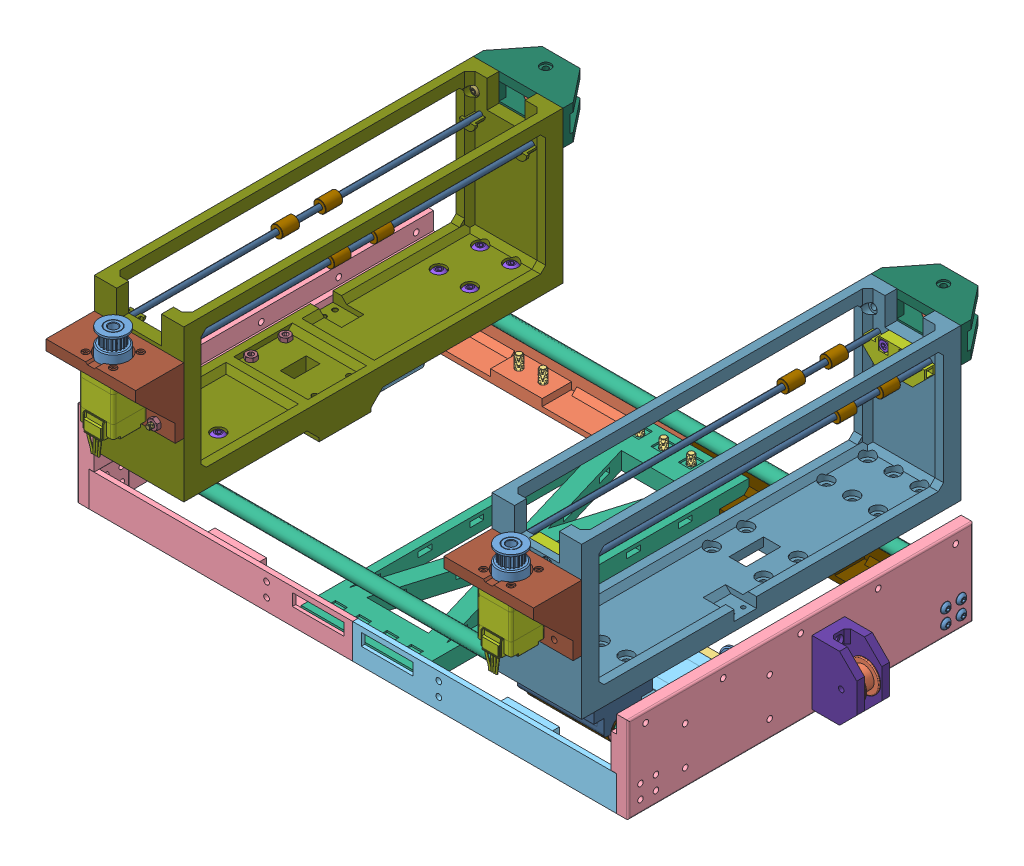
SolidWorks assembly PCBPT_V2, configuration Default. Lengths in mm.
Overall size (372.61 135 276.52).
99 component instances, 29 part files, 170 mates.
Components (placement in the parent):
- GT2_20T-1: GT2_20T [Конфигурация1] at (136.8093 1.791 -6.5027) x (0 0 1) z (-0.89688 -0.442275 0) size (16 16 16)
- GT2_toothless_bore-1: GT2_toothless_bore [Default] at (23.0237 -3.9004 33.0473) size (18 18 9)
- motor_mounting-1: motor_mounting [Default] at (119.4919 -42.7258 -9.5027) size (31.2 28.2 55)
- side_wall-1: side_wall [Default] at (109.7093 -10.1361 41.8211) x (1 0 0) z (0 1 0) size (19 200 50)
- SY28STH32-0674A-1: SY28STH32-0674A [Default] at (136.8093 1.791 -9.5027) x (1 0 0) z (0 -1 0) size (32.43 52 28.21)
- Shaft-1: Shaft [Default] at (419.7093 10.691 105.4973) x (0 1 0) z (0 0 1) size (8 300 8)
- Shaft-2: Shaft [Default] at (119.7093 10.691 -64.5027) x (0 0.381849 -0.924225) z (0 -0.924225 -0.381849) size (8 300 8)
- side_wall-2: side_wall [Default] at (429.7093 -10.1361 -0.8265) x (-1 0 0) z (0 1 0) size (19 200 50)
- SY28STH32-0674A-2: SY28STH32-0674A [Default] at (402.6093 1.791 50.4973) x (-1 0 0) z (0 -1 0) size (32.43 52 28.21)
- motor_mounting-2: motor_mounting [Default] at (419.9267 -42.7258 50.4973) x (-1 0 0) z (0 0 -1) size (31.2 28.2 55)
- GT2_toothless_bore-2: GT2_toothless_bore [Default] at (516.6229 1.0382 7.9473) x (-0.9975 -0.070666 0) z (0 0 -1) size (18 18 9)
- GT2_20T-2: GT2_20T [Конфигурация1] at (402.6093 1.791 47.4973) x (0 0 -1) z (0.794847 -0.60681 0) size (16 16 16)
- SY20STH30-0604A-3: SY20STH30-0604A [Default] at (155.7094 85.691 145.4974) x (0 0 1) z (-1 0 0) size (22.25 55.5 20.01)
- SY20STH30-0604A-4: SY20STH30-0604A [Default] at (386.4186 91.691 145.2974) x (0 0 1) z (-1 0 0) size (22.25 55.5 20.01)
- GT2_20T-3: GT2_20T [Конфигурация1] at (155.7094 88.691 145.4974) x (0 1 0) z (-0.858604 0 0.512639) size (16 16 16)
- GT2_20T-4: GT2_20T [Конфигурация1] at (386.4186 94.691 145.2974) x (0 1 0) z (-0.858604 0 0.512639) size (16 16 16)
- 94500A228_316 Stainless Steel Button Head Hex Drive Screws-1: 94500A228_316 Stainless Steel Button Head Hex Drive Screws [94500A228] at (164.7093 29.891 117.4973) x (1 0 0) z (0 1 0) size (7.6 7.6 14.61)
- 94500A228_316 Stainless Steel Button Head Hex Drive Screws-3: 94500A228_316 Stainless Steel Button Head Hex Drive Screws [94500A228] at (164.7093 29.891 93.4973) x (1 0 0) z (0 1 0) size (7.6 7.6 14.61)
- 94500A228_316 Stainless Steel Button Head Hex Drive Screws-4: 94500A228_316 Stainless Steel Button Head Hex Drive Screws [94500A228] at (146.7093 29.891 93.4973) x (1 0 0) z (0 1 0) size (7.6 7.6 14.61)
- 94500A228_316 Stainless Steel Button Head Hex Drive Screws-5: 94500A228_316 Stainless Steel Button Head Hex Drive Screws [94500A228] at (146.7093 29.891 117.4973) x (1 0 0) z (0 1 0) size (7.6 7.6 14.61)
- 94500A228_316 Stainless Steel Button Head Hex Drive Screws-6: 94500A228_316 Stainless Steel Button Head Hex Drive Screws [94500A228] at (164.7093 29.891 -76.5027) x (1 0 0) z (0 1 0) size (7.6 7.6 14.61)
- 94500A228_316 Stainless Steel Button Head Hex Drive Screws-7: 94500A228_316 Stainless Steel Button Head Hex Drive Screws [94500A228] at (164.7093 29.891 -52.5027) x (1 0 0) z (0 1 0) size (7.6 7.6 14.61)
- 94500A228_316 Stainless Steel Button Head Hex Drive Screws-8: 94500A228_316 Stainless Steel Button Head Hex Drive Screws [94500A228] at (146.7093 29.891 -76.5027) x (1 0 0) z (0 1 0) size (7.6 7.6 14.61)
- 94500A228_316 Stainless Steel Button Head Hex Drive Screws-9: 94500A228_316 Stainless Steel Button Head Hex Drive Screws [94500A228] at (146.7093 29.891 -52.5027) x (1 0 0) z (0 1 0) size (7.6 7.6 14.61)
- LM3UU-1: LM3UU [Default] at (134.6169 100.8096 0.6621) size (7 7 10)
- LM3UU-2: LM3UU [Default] at (134.6169 100.8096 25.6621) size (7 7 10)
- LM3UU-3: LM3UU [Default] at (164.6169 100.8096 0.6621) size (7 7 10)
- LM3UU-4: LM3UU [Default] at (164.6169 100.8096 25.6621) size (7 7 10)
- 3mm_shaft-1: 3mm_shaft [Default] at (138.6849 101.1199 -82.5244) size (3 3 206)
- 3mm_shaft-2: 3mm_shaft [Default] at (168.6849 101.1199 -82.5244) size (3 3 206)
- crane_motor_holder-1: crane_motor_holder [Default] at (213.6235 -30.0463 130.4973) size (52 38 28)
- 92095A119_Button Head Hex Drive Screw-1: 92095A119_Button Head Hex Drive Screw [92095A119] at (170.7093 58.691 123.8473) x (1 0 0) z (0 0 -1) size (5.7 5.7 16.99)
- 90592A085_Steel Hex Nut-1: 90592A085_Steel Hex Nut [90592A085] at (140.7093 58.691 136.6973) x (1 0 0) z (0 -1 0) size (5.5 2.79 6.35)
- 92095A119_Button Head Hex Drive Screw-2: 92095A119_Button Head Hex Drive Screw [92095A119] at (140.7093 80.691 123.8473) x (1 0 0) z (0 0 -1) size (5.7 5.7 16.99)
- 92095A119_Button Head Hex Drive Screw-3: 92095A119_Button Head Hex Drive Screw [92095A119] at (170.7093 69.691 123.8473) x (1 0 0) z (0 0 -1) size (5.7 5.7 16.99)
- 92095A119_Button Head Hex Drive Screw-4: 92095A119_Button Head Hex Drive Screw [92095A119] at (140.7093 58.691 123.8473) x (1 0 0) z (0 0 -1) size (5.7 5.7 16.99)
- 92095A119_Button Head Hex Drive Screw-5: 92095A119_Button Head Hex Drive Screw [92095A119] at (140.7093 69.691 123.8473) x (1 0 0) z (0 0 -1) size (5.7 5.7 16.99)
- 92095A119_Button Head Hex Drive Screw-6: 92095A119_Button Head Hex Drive Screw [92095A119] at (170.7093 80.691 123.8473) x (1 0 0) z (0 0 -1) size (5.7 5.7 16.99)
- 90592A085_Steel Hex Nut-2: 90592A085_Steel Hex Nut [90592A085] at (140.7093 80.691 136.6973) x (-0.923728 -0.383049 0) z (0.383049 -0.923728 0) size (5.5 2.79 6.35)
- 90592A085_Steel Hex Nut-3: 90592A085_Steel Hex Nut [90592A085] at (140.7093 69.691 136.6973) x (1 0 0) z (0 -1 0) size (5.5 2.79 6.35)
- 90592A085_Steel Hex Nut-4: 90592A085_Steel Hex Nut [90592A085] at (170.7093 80.691 136.6973) x (-0.923728 -0.383049 0) z (0.383049 -0.923728 0) size (5.5 2.79 6.35)
- 90592A085_Steel Hex Nut-5: 90592A085_Steel Hex Nut [90592A085] at (170.7093 69.691 136.6973) x (1 0 0) z (0 -1 0) size (5.5 2.79 6.35)
- 90592A085_Steel Hex Nut-6: 90592A085_Steel Hex Nut [90592A085] at (170.7093 58.691 136.6973) x (1 0 0) z (0 -1 0) size (5.5 2.79 6.35)
- crane2-2: crane2 [Default] at (352.6573 27.691 -36.7605) size (52 88 220)
- crane_motor_holder-2: crane_motor_holder [Default] at (444.3326 -24.0463 130.2973) size (52 38 28)
- 3mm_shaft-3: 3mm_shaft [Default] at (369.394 107.1199 -82.7027) size (3 3 206)
- 3mm_shaft-4: 3mm_shaft [Default] at (399.394 107.1199 -82.7027) size (3 3 206)
- LM3UU-5: LM3UU [Default] at (365.326 106.8096 -62.3076) size (7 7 10)
- LM3UU-6: LM3UU [Default] at (395.326 106.8096 -62.3076) size (7 7 10)
- LM3UU-7: LM3UU [Default] at (365.326 106.8096 -37.3076) size (7 7 10)
- LM3UU-8: LM3UU [Default] at (395.326 106.8096 -37.3076) size (7 7 10)
- GT2_toothless_bore-3: GT2_toothless_bore [Default] at (443.5602 109.141 -65.4124) x (-0.861467 0 -0.507814) z (0 -1 0) size (18 18 9)
- GT2_toothless_bore-4: GT2_toothless_bore [Default] at (217.7831 103.141 -73.3261) x (-0.922327 0 -0.38641) z (0 -1 0) size (18 18 9)
- crane_noteeth_pulley_holder-1: crane_noteeth_pulley_holder [Default] at (-128.1118 -24.7792 -114.7027) size (52 20 25)
- crane_noteeth_pulley_holder-2: crane_noteeth_pulley_holder [Default] at (-358.821 -30.7792 -114.5027) size (52 20 25)
- 92095A119_Button Head Hex Drive Screw-7: 92095A119_Button Head Hex Drive Screw [92095A119] at (137.2093 99.691 -81.8527) x (-0.992337 0.123563 0) z (0 0 1) size (5.7 5.7 16.99)
- 92095A119_Button Head Hex Drive Screw-8: 92095A119_Button Head Hex Drive Screw [92095A119] at (174.2093 99.691 -81.8527) x (-0.992337 0.123563 0) z (0 0 1) size (5.7 5.7 16.99)
- 90592A085_Steel Hex Nut-7: 90592A085_Steel Hex Nut [90592A085] at (137.2093 99.691 -93.7027) x (1 0 0) z (0 -1 0) size (5.5 2.79 6.35)
- 90592A085_Steel Hex Nut-8: 90592A085_Steel Hex Nut [90592A085] at (174.2093 99.691 -93.7027) x (1 0 0) z (0 -1 0) size (5.5 2.79 6.35)
- crane1-1: crane1 [Default] at (121.9481 21.691 -36.5654) size (52 97 220)
- toothless_pulley_mount-3: toothless_pulley_mount [Default] at (148.31 -14.1951 27.0473) x (-1 0 0) z (0 1 0) size (26 19 37.2)
- toothless_pulley_mount-4: toothless_pulley_mount [Default] at (391.1086 -14.1951 13.9473) x (1 0 0) z (0 1 0) size (26 19 37.2)
- 90592A085_Steel Hex Nut-10: 90592A085_Steel Hex Nut [90592A085] at (174.2093 30.891 26.9924) x (-1 0 0) z (0 0 -1) size (5.5 2.79 6.35) (hidden)
- 90592A085_Steel Hex Nut-11: 90592A085_Steel Hex Nut [90592A085] at (137.2093 30.891 26.9924) x (1 0 0) z (0 0 -1) size (5.5 2.79 6.35)
- 90592A085_Steel Hex Nut-12: 90592A085_Steel Hex Nut [90592A085] at (137.2093 30.891 46.9924) x (-0.5 0 -0.866025) z (0.866025 0 -0.5) size (5.5 2.79 6.35)
- frame1-2: frame1 [Default] at (511.1109 22.8663 -76.5027) x (-1 0 0) z (0 0 -1) size (153 20 20)
- 90592A085_Steel Hex Nut-17: 90592A085_Steel Hex Nut [90592A085] at (418.5093 -12.309 -72.5027) x (0 0.965926 -0.258819) z (0 -0.258819 -0.965926) size (5.5 2.79 6.35)
- 90592A085_Steel Hex Nut-18: 90592A085_Steel Hex Nut [90592A085] at (418.5093 -4.309 -72.5027) x (0 0.608045 -0.793903) z (0 0.793903 0.608045) size (5.5 2.79 6.35)
- 90592A085_Steel Hex Nut-19: 90592A085_Steel Hex Nut [90592A085] at (418.5093 -4.309 -63.5027) x (0 0.965926 -0.258819) z (0 -0.258819 -0.965926) size (5.5 2.79 6.35)
- 90592A085_Steel Hex Nut-20: 90592A085_Steel Hex Nut [90592A085] at (418.5093 -12.309 -63.5027) x (0 0.608045 -0.793903) z (0 0.793903 0.608045) size (5.5 2.79 6.35)
- 92095A168_Button Head Hex Drive Screw-1: 92095A168_Button Head Hex Drive Screw [92095A168] at (431.3593 -4.309 -63.5027) x (0 0 -1) z (1 0 0) size (5.7 5.7 15.99)
- 92095A168_Button Head Hex Drive Screw-2: 92095A168_Button Head Hex Drive Screw [92095A168] at (431.3593 -12.309 -63.5027) x (0 0 -1) z (1 0 0) size (5.7 5.7 15.99)
- 92095A168_Button Head Hex Drive Screw-3: 92095A168_Button Head Hex Drive Screw [92095A168] at (431.3593 -12.309 -72.5027) x (0 0 -1) z (1 0 0) size (5.7 5.7 15.99)
- 92095A168_Button Head Hex Drive Screw-4: 92095A168_Button Head Hex Drive Screw [92095A168] at (431.3593 -4.309 -72.5027) x (0 0 -1) z (1 0 0) size (5.7 5.7 15.99)
- frame2-2: frame2 [Default] at (119.7093 0.1922 28.7428) x (-1 0 0) z (0 0 -1) size (153 20 20)
- 92095A192_Button Head Hex Drive Screw-1: 92095A192_Button Head Hex Drive Screw [92095A192] at (291.7093 -19.009 -68.0027) x (1 0 0) z (0 -1 0) size (7.6 7.6 14.61)
- 92095A192_Button Head Hex Drive Screw-2: 92095A192_Button Head Hex Drive Screw [92095A192] at (277.7093 -19.009 -68.0027) x (1 0 0) z (0 -1 0) size (7.6 7.6 14.61)
- 92095A192_Button Head Hex Drive Screw-3: 92095A192_Button Head Hex Drive Screw [92095A192] at (361.7093 -19.009 -68.0027) x (1 0 0) z (0 -1 0) size (7.6 7.6 14.61)
- 92095A192_Button Head Hex Drive Screw-4: 92095A192_Button Head Hex Drive Screw [92095A192] at (347.7093 -19.009 -68.0027) x (1 0 0) z (0 -1 0) size (7.6 7.6 14.61)
- 92095A192_Button Head Hex Drive Screw-5: 92095A192_Button Head Hex Drive Screw [92095A192] at (261.7093 -19.009 -68.0027) x (1 0 0) z (0 -1 0) size (7.6 7.6 14.61)
- 92095A192_Button Head Hex Drive Screw-6: 92095A192_Button Head Hex Drive Screw [92095A192] at (247.7093 -19.009 -68.0027) x (1 0 0) z (0 -1 0) size (7.6 7.6 14.61)
- 92095A192_Button Head Hex Drive Screw-7: 92095A192_Button Head Hex Drive Screw [92095A192] at (191.7093 -19.009 -68.0027) x (1 0 0) z (0 -1 0) size (7.6 7.6 14.61)
- 92095A192_Button Head Hex Drive Screw-8: 92095A192_Button Head Hex Drive Screw [92095A192] at (177.7093 -19.009 -68.0027) x (1 0 0) z (0 -1 0) size (7.6 7.6 14.61)
- frame3-1: frame3 [Default] at (28.3077 22.8663 117.4973) size (153 20 20)
- frame4-1: frame4 [Default] at (419.7093 0.1922 12.2519) size (153 20 20)
- frame5-1: frame5 [Default] at (55.0941 -19.309 10.0347) size (66 10 193.8)
- frame6-1: frame6 [Default] at origin
- crane_shaft_holder-1: crane_shaft_holder [Default] at (46.8369 7.7409 -82.7027) size (36 16 6)
- 91828A211_18-8 Stainless Steel Hex Nut-1: 91828A211_18-8 Stainless Steel Hex Nut [91828A211] at (380.4185 95.691 -78.1027) size (5.5 6.35 2.78)
- 91828A211_18-8 Stainless Steel Hex Nut-2: 91828A211_18-8 Stainless Steel Hex Nut [91828A211] at (392.4185 95.691 -78.1027) x (-1 0 0) z (0 0 -1) size (5.5 6.35 2.78)
- 91828A211_18-8 Stainless Steel Hex Nut-3: 91828A211_18-8 Stainless Steel Hex Nut [91828A211] at (386.4185 87.691 -78.1027) x (-1 0 0) z (0 0 -1) size (5.5 6.35 2.78)
- crane_shaft_holder-2: crane_shaft_holder [Default] at (726.0001 7.7409 126.1693) x (-1 0 0) z (0 0 -1) size (36 16 6)
- 91828A211_18-8 Stainless Steel Hex Nut-4: 91828A211_18-8 Stainless Steel Hex Nut [91828A211] at (380.4185 95.691 121.5693) size (5.5 6.35 2.78)
- 91828A211_18-8 Stainless Steel Hex Nut-5: 91828A211_18-8 Stainless Steel Hex Nut [91828A211] at (392.4185 95.691 121.5693) size (5.5 6.35 2.78)
- 91828A211_18-8 Stainless Steel Hex Nut-6: 91828A211_18-8 Stainless Steel Hex Nut [91828A211] at (386.4185 87.691 121.5693) size (5.5 6.35 2.78)
- LM8UU_double_holder-1: LM8UU_double_holder [Default] at (403.779 7.5927 131.4203) x (0 0 -1) z (1 0 0) size (34 24.51 50)
  - Lm8uu-2: Lm8uu [Default] at (25.923 3.0983 -5.3605) size (15 15 24)
  - holder_1-1: holder_1 [Default] at (15.1975 13.0983 -7.3181) size (34 17.01 50)
  - Lm8uu-3: Lm8uu [Default] at (25.923 3.0983 -29.3605) size (15 15 24)
Mates (geometry in assembly coordinates):
- Concentric2: concentric anti-aligned: cylinder of motor_mounting-1 through (136.8093 1.791 -9.5027) axis (0 0 1) radius 11.5; cylinder of SY28STH32-0674A-1 through (136.8093 1.791 -7.5027) axis (0 0 -1) radius 11
- Coincident2: coincident anti-aligned: plane of motor_mounting-1 through (119.4919 -42.7258 -9.5027) normal (0 0 -1); plane of SY28STH32-0674A-1 through (136.8093 1.791 -9.5027) normal (0 0 1)
- Distance1: distance = 1 mm anti-aligned: plane of GT2_20T-1 through (136.8093 1.791 -6.5027) normal (0 0 -1); plane of SY28STH32-0674A-1 through (136.8093 1.791 -7.5027) normal (0 0 1)
- Concentric4: concentric anti-aligned: cylinder of GT2_20T-1 through (136.8093 1.791 -6.5027) axis (0 0 1) radius 2.5; cylinder of SY28STH32-0674A-1 through (136.8093 1.791 10.4973) axis (0 0 -1) radius 2.5
- Distance7: distance = 21.1 mm: cylinder of GT2_toothless_bore-1 through (92.7093 1.791 40.0473) axis (0 0 -1) radius 6.05; plane of side_wall-1 through (119.7093 -19.309 -79.5027) normal (0 -1 0)
- Coincident11: coincident anti-aligned: plane of side_wall-1 through (119.7093 -10.1361 41.8211) normal (1 0 0); plane of Shaft-2 through (119.7093 10.691 -64.5027) normal (-1 0 0)
- Coincident16: coincident anti-aligned: plane of SY28STH32-0674A-2 through (416.7092 -12.3089 75.2473) normal (1 0 0); plane of motor_mounting-2 through (416.7093 -42.7258 50.4973) normal (-1 0 0)
- Concentric14: concentric anti-aligned: cylinder of SY28STH32-0674A-2 through (402.6093 1.791 48.4973) axis (0 0 1) radius 11; cylinder of motor_mounting-2 through (402.6093 1.791 50.4973) axis (0 0 -1) radius 11.5
- Coincident17: coincident anti-aligned: plane of SY28STH32-0674A-2 through (402.6093 1.791 50.4973) normal (0 0 -1); plane of motor_mounting-2 through (419.9267 -42.7258 50.4973) normal (0 0 1)
- Coincident18: coincident anti-aligned: plane of side_wall-2 through (419.7093 -10.1361 -0.8265) normal (-1 0 0); plane of motor_mounting-2 through (419.7093 -42.7258 50.4973) normal (1 0 0)
- Distance8: distance = 87.45 mm aligned: plane of GT2_toothless_bore-1 through (92.7093 1.791 33.0473) normal (0 0 1); plane of side_wall-1 through (119.7093 30.691 120.4973) normal (0 0 1)
- Concentric19: concentric aligned: cylinder of SY28STH32-0674A-2 through (402.6093 1.791 30.4973) axis (0 0 1) radius 2.5; cylinder of GT2_20T-2 through (402.6093 1.791 47.4973) axis (0 0 1) radius 8
- Distance10: distance = 1 mm anti-aligned: plane of GT2_20T-2 through (402.6093 1.791 47.4973) normal (0 0 1); plane of SY28STH32-0674A-2 through (402.6093 1.791 48.4973) normal (0 0 -1)
- Coincident33: coincident anti-aligned: plane of motor_mounting-1 through (119.7093 -42.7258 -9.5027) normal (-1 0 0); plane of side_wall-1 through (119.7093 -10.1361 41.8211) normal (1 0 0)
- Distance26: distance = 7 mm aligned: plane of motor_mounting-1 through (122.7093 -12.309 -4.5027) normal (0 -1 0); plane of side_wall-1 through (119.7093 -19.309 -79.5027) normal (0 -1 0)
- Concentric29: concentric anti-aligned: cylinder of SY20STH30-0604A-3 through (155.7094 100.691 145.4974) axis (0 -1 0) radius 2; cylinder of GT2_20T-3 through (155.7094 88.691 145.4974) axis (0 1 0) radius 2.5
- Coincident35: coincident anti-aligned: plane of SY20STH30-0604A-3 through (155.7094 88.691 145.4974) normal (0 1 0); plane of GT2_20T-3 through (155.7094 88.691 145.4974) normal (0 -1 0)
- Concentric30: concentric anti-aligned: cylinder of SY20STH30-0604A-4 through (386.4186 106.691 145.2974) axis (0 -1 0) radius 2; cylinder of GT2_20T-4 through (386.4186 94.691 145.2974) axis (0 1 0) radius 2.5
- Coincident36: coincident anti-aligned: plane of SY20STH30-0604A-4 through (386.4186 94.691 145.2974) normal (0 1 0); plane of GT2_20T-4 through (386.4186 94.691 145.2974) normal (0 -1 0)
- Concentric31: concentric aligned: cylinder of Shaft-2 through (419.7093 10.691 -64.5027) axis (-1 0 0) radius 4; cylinder of side_wall-2 through (431.1644 10.691 -64.5027) axis (-1 0 0) radius 4.05
- Coincident37: coincident aligned: plane of motor_mounting-1 through (122.7093 -12.309 -4.5027) normal (0 -1 0); plane of motor_mounting-2 through (416.7093 -12.309 45.4973) normal (0 -1 0)
- Distance27: distance = 30 mm aligned: plane of motor_mounting-2 through (419.7093 15.891 90.4973) normal (0 0 1); plane of side_wall-2 through (419.7093 30.691 120.4973) normal (0 0 1)
- Coincident39: coincident anti-aligned: plane of side_wall-2 through (419.7093 -10.1361 -0.8265) normal (-1 0 0); plane of motor_mounting-2 through (419.7093 -42.7258 50.4973) normal (1 0 0)
- Distance40: distance = 30 mm aligned: plane of motor_mounting-1 through (119.7093 15.891 -49.5027) normal (0 0 -1); plane of side_wall-1 through (119.7093 30.691 -79.5027) normal (0 0 -1)
- Coincident113: coincident aligned: plane of 94500A228_316 Stainless Steel Button Head Hex Drive Screws-6 through (160.8993 27.691 -72.7027) normal (0 -1 0); plane of 94500A228_316 Stainless Steel Button Head Hex Drive Screws-7 through (160.8993 27.691 -48.7027) normal (0 -1 0)
- Concentric69: concentric aligned: cylinder of LM3UU-1 through (140.7093 89.691 10.6621) axis (0 0 -1) radius 3.5; cylinder of LM3UU-2 through (140.7093 89.691 35.6621) axis (0 0 -1) radius 3.5
- Concentric70: concentric aligned: cylinder of LM3UU-3 through (170.7093 89.691 10.6621) axis (0 0 -1) radius 3.5; cylinder of LM3UU-4 through (170.7093 89.691 35.6621) axis (0 0 -1) radius 3.5
- Concentric73: concentric aligned: cylinder of LM3UU-2 through (140.7093 89.691 35.6621) axis (0 0 -1) radius 3.5; cylinder of 3mm_shaft-1 through (140.7093 89.691 123.4756) axis (0 0 -1) radius 1.5
- Concentric74: concentric aligned: cylinder of LM3UU-4 through (170.7093 89.691 35.6621) axis (0 0 -1) radius 3.5; cylinder of 3mm_shaft-2 through (170.7093 89.691 123.4756) axis (0 0 -1) radius 1.5
- Coincident131: coincident anti-aligned: plane of SY20STH30-0604A-3 through (145.7093 64.691 135.4973) normal (0 0 -1); plane of crane_motor_holder-1 through (213.6235 -30.0463 135.4973) normal (0 0 1)
- Coincident132: coincident anti-aligned: plane of SY20STH30-0604A-3 through (155.7094 85.691 145.4974) normal (0 1 0); plane of crane_motor_holder-1 through (129.7093 85.691 158.4973) normal (0 -1 0)
- Parallel1: parallel anti-aligned: cylinder of SY20STH30-0604A-3 through (147.7094 82.191 153.4974) axis (0 1 0) radius 1; cylinder of crane_motor_holder-1 through (147.7094 94.9436 153.4974) axis (0 -1 0) radius 1.15
- Coincident141: coincident anti-aligned: plane of crane_motor_holder-1 through (213.6235 -30.0463 135.4973) normal (0 0 1); plane of 90592A085_Steel Hex Nut-1 through (137.9593 60.2787 135.4973) normal (0 0 -1)
- Concentric82: concentric aligned: circle of crane_motor_holder-1; circle of 90592A085_Steel Hex Nut-1
- Coincident1431: coincident anti-aligned: plane of crane_motor_holder-1 through (213.6235 -30.0463 135.4973) normal (0 0 1); plane of 90592A085_Steel Hex Nut-3 through (137.9593 71.2787 135.4973) normal (0 0 -1)
- Coincident1441: coincident anti-aligned: plane of crane_motor_holder-1 through (213.6235 -30.0463 135.4973) normal (0 0 1); plane of 90592A085_Steel Hex Nut-4 through (172.6414 83.211 135.4973) normal (0 0 -1)
- Coincident1451: coincident anti-aligned: plane of crane_motor_holder-1 through (213.6235 -30.0463 135.4973) normal (0 0 1); plane of 90592A085_Steel Hex Nut-5 through (167.9593 71.2787 135.4973) normal (0 0 -1)
- Coincident1461: coincident anti-aligned: plane of crane_motor_holder-1 through (213.6235 -30.0463 135.4973) normal (0 0 1); plane of 90592A085_Steel Hex Nut-6 through (167.9593 60.2787 135.4973) normal (0 0 -1)
- Concentric83: concentric anti-aligned: circle of crane_motor_holder-1; circle of 90592A085_Steel Hex Nut-2
- Concentric84: concentric aligned: circle of crane_motor_holder-1; circle of 90592A085_Steel Hex Nut-3
- Concentric85: concentric anti-aligned: circle of crane_motor_holder-1; circle of 90592A085_Steel Hex Nut-4
- Concentric86: concentric aligned: circle of crane_motor_holder-1; circle of 90592A085_Steel Hex Nut-5
- Concentric87: concentric aligned: circle of crane_motor_holder-1; circle of 90592A085_Steel Hex Nut-6
- Coincident160: coincident anti-aligned: plane of crane2-2 through (360.4185 35.691 130.2973) normal (0 0 1); plane of crane_motor_holder-2 through (444.3326 -24.0463 130.2973) normal (0 0 -1)
- Concentric99: concentric aligned: cylinder of crane2-2 through (371.4185 64.691 120.2973) axis (0 0 1) radius 1.65; cylinder of crane_motor_holder-2 through (371.4185 64.691 130.2973) axis (0 0 1) radius 1.65
- Coincident161: coincident anti-aligned: plane of SY20STH30-0604A-4 through (376.4185 70.691 135.2973) normal (0 0 -1); plane of crane_motor_holder-2 through (444.3326 -24.0463 135.2973) normal (0 0 1)
- Coincident162: coincident anti-aligned: plane of SY20STH30-0604A-4 through (386.4186 91.691 145.2974) normal (0 1 0); plane of crane_motor_holder-2 through (360.4185 91.691 158.2973) normal (0 -1 0)
- Concentric100: concentric anti-aligned: cylinder of SY20STH30-0604A-4 through (378.4186 88.191 153.2974) axis (0 1 0) radius 1; cylinder of crane_motor_holder-2 through (378.4186 100.9436 153.2974) axis (0 -1 0) radius 1.15
- Coincident171: coincident anti-aligned: plane of crane2-2 through (412.4185 115.691 -82.7027) normal (0 0 1); plane of 3mm_shaft-4 through (401.4185 95.691 -82.7027) normal (0 0 -1)
- Coincident172: coincident anti-aligned: plane of crane2-2 through (412.4185 115.691 -82.7027) normal (0 0 1); plane of 3mm_shaft-3 through (371.4185 95.691 -82.7027) normal (0 0 -1)
- Concentric111: concentric aligned: cylinder of 3mm_shaft-4 through (401.4185 95.691 123.2973) axis (0 0 -1) radius 1.5; cylinder of LM3UU-6 through (401.4185 95.691 -52.3076) axis (0 0 -1) radius 3.5
- Concentric112: concentric aligned: cylinder of 3mm_shaft-4 through (401.4185 95.691 123.2973) axis (0 0 -1) radius 1.5; cylinder of LM3UU-8 through (401.4185 95.691 -27.3076) axis (0 0 -1) radius 3.5
- Concentric113: concentric aligned: cylinder of 3mm_shaft-3 through (371.4185 95.691 123.2973) axis (0 0 -1) radius 1.5; cylinder of LM3UU-5 through (371.4185 95.691 -52.3076) axis (0 0 -1) radius 3.5
- Concentric114: concentric aligned: cylinder of 3mm_shaft-3 through (371.4185 95.691 123.2973) axis (0 0 -1) radius 1.5; cylinder of LM3UU-7 through (371.4185 95.691 -27.3076) axis (0 0 -1) radius 3.5
- Parallel5: parallel aligned: plane of crane2-2 through (352.6573 115.691 -36.7605) normal (0 1 0); plane of GT2_toothless_bore-3 through (386.4185 110.141 -105.7027) normal (0 1 0)
- Coincident1464: coincident aligned: plane of GT2_20T-4 through (386.4186 102.141 145.2974) normal (0 1 0); plane of GT2_toothless_bore-3 through (386.4185 102.141 -105.7027) normal (0 1 0)
- Coincident1465: coincident aligned: plane of GT2_20T-3 through (155.7094 96.141 145.4974) normal (0 1 0); plane of GT2_toothless_bore-4 through (155.7093 96.141 -105.5027) normal (0 1 0)
- Coincident1466: coincident anti-aligned: plane of crane2-2 through (360.4185 35.691 -89.7027) normal (0 0 -1); plane of crane_noteeth_pulley_holder-1 through (-128.1118 -24.7792 -89.7027) normal (0 0 1)
- Coincident1467: coincident aligned: plane of crane2-2 through (412.4185 35.691 -89.7027) normal (1 0 0); plane of crane_noteeth_pulley_holder-1 through (412.4185 115.691 -89.7027) normal (1 0 0)
- Coincident1468: coincident aligned: plane of crane2-2 through (352.6573 115.691 -36.7605) normal (0 1 0); plane of crane_noteeth_pulley_holder-1 through (412.4185 115.691 -89.7027) normal (0 1 0)
- Concentric115: concentric aligned: circle of GT2_toothless_bore-3; cylinder of crane_noteeth_pulley_holder-1 through (386.4185 94.1438 -105.7027) axis (0 1 0) radius 1.6
- Concentric116: concentric aligned: cylinder of GT2_toothless_bore-4 through (155.7093 95.141 -105.5027) axis (0 1 0) radius 1.5; cylinder of crane_noteeth_pulley_holder-2 through (155.7093 89.691 -105.5027) axis (0 1 0) radius 1.6
- Coincident1475: coincident anti-aligned: plane of crane_noteeth_pulley_holder-2 through (-358.821 -30.7792 -92.5027) normal (0 0 -1); plane of 90592A085_Steel Hex Nut-7 through (134.4593 101.2787 -92.5027) normal (0 0 1)
- Concentric120: concentric anti-aligned: cylinder of crane_noteeth_pulley_holder-2 through (137.2093 99.691 -89.5027) axis (0 0 -1) radius 1.6; circle of 90592A085_Steel Hex Nut-7
- Coincident1476: coincident anti-aligned: plane of crane_noteeth_pulley_holder-2 through (-358.821 -30.7792 -92.5027) normal (0 0 -1); plane of 90592A085_Steel Hex Nut-8 through (171.4593 101.2787 -92.5027) normal (0 0 1)
- Concentric121: concentric anti-aligned: cylinder of crane_noteeth_pulley_holder-2 through (174.2093 99.691 -89.5027) axis (0 0 -1) radius 1.6; circle of 90592A085_Steel Hex Nut-8
- Distance43: distance = 15 mm anti-aligned: plane of LM3UU-1 through (140.7093 89.691 10.6621) normal (0 0 1); plane of LM3UU-2 through (140.7093 89.691 25.6621) normal (0 0 -1)
- Coincident1478: coincident aligned: plane of LM3UU-2 through (140.7093 89.691 35.6621) normal (0 0 1); plane of LM3UU-4 through (170.7093 89.691 35.6621) normal (0 0 1)
- Coincident1479: coincident aligned: plane of LM3UU-1 through (140.7093 89.691 10.6621) normal (0 0 1); plane of LM3UU-3 through (170.7093 89.691 10.6621) normal (0 0 1)
- Coincident1480: coincident anti-aligned: plane of crane_motor_holder-1 through (213.6235 -30.0463 135.4973) normal (0 0 1); plane of 90592A085_Steel Hex Nut-2 through (142.6414 83.211 135.4973) normal (0 0 -1)
- Coincident1484: coincident aligned: plane of crane2-2 through (360.4185 35.691 -89.7027) normal (-1 0 0); plane of crane_motor_holder-2 through (360.4185 97.691 135.2973) normal (-1 0 0)
- Parallel6: parallel anti-aligned: plane of crane2-2 through (360.4185 35.691 -89.7027) normal (-1 0 0); plane of crane1-1 through (181.7093 29.691 -89.5076) normal (1 0 0)
- Concentric122: concentric aligned: cylinder of crane_noteeth_pulley_holder-2 through (174.2093 99.691 -89.5027) axis (0 0 -1) radius 1.6; cylinder of crane1-1 through (174.2093 99.691 -79.5076) axis (0 0 -1) radius 1.65
- Coincident1485: coincident anti-aligned: plane of side_wall-1 through (109.7093 -10.1361 41.8211) normal (-1 0 0); plane of toothless_pulley_mount-3 through (109.7093 20.391 46.0473) normal (1 0 0)
- Concentric125: concentric aligned: cylinder of GT2_toothless_bore-1 through (92.7093 1.791 41.0473) axis (0 0 -1) radius 1.5; cylinder of toothless_pulley_mount-3 through (92.7093 1.791 46.0473) axis (0 0 -1) radius 1.6
- Distance44: distance = 0.5 mm anti-aligned: plane of toothless_pulley_mount-3 through (83.7093 -16.809 41.5473) normal (0 0 -1); plane of GT2_toothless_bore-1 through (92.7093 1.791 41.0473) normal (0 0 1)
- Coincident1491: coincident anti-aligned: plane of side_wall-2 through (429.7093 -10.1361 -0.8265) normal (1 0 0); plane of toothless_pulley_mount-4 through (429.7093 20.391 -5.0527) normal (-1 0 0)
- Coincident1492: coincident aligned: plane of side_wall-2 through (429.7093 12.891 9.4473) normal (0 0 -1); plane of toothless_pulley_mount-4 through (455.7093 -16.809 9.4473) normal (0 0 -1)
- Coincident1493: coincident aligned: plane of side_wall-2 through (429.7093 12.891 -0.5527) normal (0 -1 0); plane of toothless_pulley_mount-4 through (429.7093 12.891 9.4473) normal (0 -1 0)
- Concentric126: concentric aligned: cylinder of GT2_toothless_bore-2 through (446.7093 1.791 -0.0527) axis (0 0 1) radius 1.5; cylinder of toothless_pulley_mount-4 through (446.7093 1.791 -5.0527) axis (0 0 1) radius 1.6
- Distance47: distance = 87.45 mm aligned: plane of GT2_toothless_bore-2 through (446.7093 1.791 7.9473) normal (0 0 -1); plane of side_wall-2 through (419.7093 30.691 -79.5027) normal (0 0 -1)
- Coincident14961: coincident anti-aligned: plane of crane1-1 through (121.9481 29.691 -36.5654) normal (0 1 0); plane of 90592A085_Steel Hex Nut-10 through (176.9593 29.691 28.5801) normal (0 -1 0)
- Coincident14971: coincident anti-aligned: plane of crane1-1 through (121.9481 29.691 -36.5654) normal (0 1 0); plane of 90592A085_Steel Hex Nut-11 through (134.4593 29.691 28.5801) normal (0 -1 0)
- Coincident14981: coincident anti-aligned: plane of crane1-1 through (121.9481 29.691 -36.5654) normal (0 1 0); plane of 90592A085_Steel Hex Nut-12 through (137.2093 29.691 50.1679) normal (0 -1 0)
- Concentric128: concentric aligned: cylinder of crane1-1 through (137.2093 37.2164 26.9924) axis (0 -1 0) radius 1.6; circle of 90592A085_Steel Hex Nut-11
- Concentric129: concentric anti-aligned: cylinder of crane1-1 through (137.2093 37.2164 46.9924) axis (0 -1 0) radius 1.6; circle of 90592A085_Steel Hex Nut-12
- Parallel12: parallel anti-aligned: plane of crane1-1 through (134.2093 67.4041 19.9924) normal (1 0 0); plane of 90592A085_Steel Hex Nut-12 through (134.4593 32.091 45.4047) normal (-1 0 0)
- Concentric130: concentric anti-aligned: cylinder of crane1-1 through (174.2093 37.2164 26.9924) axis (0 -1 0) radius 1.6; circle of 90592A085_Steel Hex Nut-10
- Parallel13: parallel anti-aligned: plane of crane1-1 through (177.2093 67.4041 19.9924) normal (-1 0 0); plane of 90592A085_Steel Hex Nut-10 through (176.9593 32.091 28.5801) normal (1 0 0)
- Distance48: distance = 15 mm anti-aligned: plane of LM3UU-5 through (371.4185 95.691 -52.3076) normal (0 0 1); plane of LM3UU-7 through (371.4185 95.691 -37.3076) normal (0 0 -1)
- Distance49: distance = 15 mm anti-aligned: plane of LM3UU-8 through (401.4185 95.691 -37.3076) normal (0 0 -1); plane of LM3UU-6 through (401.4185 95.691 -52.3076) normal (0 0 1)
- Coincident1509: coincident aligned: plane of LM3UU-7 through (371.4185 95.691 -27.3076) normal (0 0 1); plane of LM3UU-8 through (401.4185 95.691 -27.3076) normal (0 0 1)
- Coincident15045: coincident anti-aligned: plane of side_wall-2 through (422.7093 -10.1361 -0.8265) normal (-1 0 0); plane of frame1-2 through (422.7093 0.691 -79.5027) normal (1 0 0)
- Coincident15046: coincident aligned: plane of side_wall-2 through (419.7093 -19.309 120.4973) normal (0 -1 0); plane of frame1-2 through (422.7093 -19.309 -79.5027) normal (0 -1 0)
- Coincident15047: coincident aligned: plane of side_wall-2 through (419.7093 30.691 -79.5027) normal (0 0 -1); plane of frame1-2 through (511.1109 22.8663 -79.5027) normal (0 0 -1)
- Coincident15048: coincident anti-aligned: plane of frame1-2 through (419.7093 0.691 -59.5027) normal (-1 0 0); plane of 90592A085_Steel Hex Nut-17 through (419.7093 -14.5544 -70.2573) normal (1 0 0)
- Concentric135: concentric aligned: circle of frame1-2; circle of 90592A085_Steel Hex Nut-17
- Coincident150511: coincident anti-aligned: plane of frame1-2 through (419.7093 0.691 -59.5027) normal (-1 0 0); plane of 90592A085_Steel Hex Nut-18 through (419.7093 -7.2417 -71.2848) normal (1 0 0)
- Concentric136: concentric anti-aligned: circle of frame1-2; circle of 90592A085_Steel Hex Nut-18
- Coincident150521: coincident anti-aligned: plane of frame1-2 through (419.7093 0.691 -59.5027) normal (-1 0 0); plane of 90592A085_Steel Hex Nut-19 through (419.7093 -6.5544 -61.2573) normal (1 0 0)
- Coincident150531: coincident anti-aligned: plane of frame1-2 through (419.7093 0.691 -59.5027) normal (-1 0 0); plane of 90592A085_Steel Hex Nut-20 through (419.7093 -15.2417 -62.2848) normal (1 0 0)
- Concentric137: concentric aligned: circle of frame1-2; circle of 90592A085_Steel Hex Nut-19
- Concentric138: concentric anti-aligned: circle of frame1-2; circle of 90592A085_Steel Hex Nut-20
- Coincident15054: coincident anti-aligned: plane of side_wall-2 through (429.7093 -10.1361 -0.8265) normal (1 0 0); plane of 92095A168_Button Head Hex Drive Screw-1 through (429.7093 -4.309 -66.3527) normal (-1 0 0)
- Concentric139: concentric anti-aligned: circle of side_wall-2; circle of 92095A168_Button Head Hex Drive Screw-1
- Coincident15055: coincident anti-aligned: plane of side_wall-2 through (429.7093 -10.1361 -0.8265) normal (1 0 0); plane of 92095A168_Button Head Hex Drive Screw-2 through (429.7093 -12.309 -66.3527) normal (-1 0 0)
- Concentric140: concentric anti-aligned: cylinder of side_wall-2 through (429.7093 -12.309 -63.5027) axis (-1 0 0) radius 1.6; circle of 92095A168_Button Head Hex Drive Screw-2
- Coincident15056: coincident anti-aligned: plane of side_wall-2 through (429.7093 -10.1361 -0.8265) normal (1 0 0); plane of 92095A168_Button Head Hex Drive Screw-4 through (429.7093 -4.309 -75.3527) normal (-1 0 0)
- Concentric141: concentric anti-aligned: cylinder of side_wall-2 through (429.7093 -4.309 -72.5027) axis (-1 0 0) radius 1.6; circle of 92095A168_Button Head Hex Drive Screw-4
- Coincident15057: coincident anti-aligned: plane of side_wall-2 through (429.7093 -10.1361 -0.8265) normal (1 0 0); plane of 92095A168_Button Head Hex Drive Screw-3 through (429.7093 -12.309 -75.3527) normal (-1 0 0)
- Concentric142: concentric anti-aligned: cylinder of side_wall-2 through (429.7093 -12.309 -72.5027) axis (-1 0 0) radius 1.6; circle of 92095A168_Button Head Hex Drive Screw-3
- Coincident150536: coincident anti-aligned: plane of side_wall-1 through (116.7093 -10.1361 41.8211) normal (1 0 0); plane of frame2-2 through (116.7093 0.1922 28.7428) normal (-1 0 0)
- Coincident150537: coincident aligned: plane of side_wall-1 through (119.7093 30.691 -79.5027) normal (0 0 -1); plane of frame2-2 through (116.7093 0.691 -79.5027) normal (0 0 -1)
- Coincident150538: coincident aligned: plane of side_wall-1 through (119.7093 -19.309 -79.5027) normal (0 -1 0); plane of frame2-2 through (116.7093 -19.309 -59.5027) normal (0 -1 0)
- Concentric151: concentric anti-aligned: cylinder of 3mm_shaft-1 through (140.7093 89.691 123.4756) axis (0 0 -1) radius 1.5; cylinder of crane1-1 through (140.7093 89.691 -86.8916) axis (0 0 1) radius 1.55
- Concentric152: concentric anti-aligned: cylinder of 3mm_shaft-2 through (170.7093 89.691 123.4756) axis (0 0 -1) radius 1.5; cylinder of crane1-1 through (170.7093 89.691 -86.8916) axis (0 0 1) radius 1.55
- Coincident150539: coincident anti-aligned: plane of frame1-2 through (291.7093 -16.809 -68.0027) normal (0 -1 0); plane of 92095A192_Button Head Hex Drive Screw-1 through (295.5093 -16.809 -68.0027) normal (0 1 0)
- Concentric153: concentric anti-aligned: cylinder of frame1-2 through (291.7093 -19.309 -68.0027) axis (0 1 0) radius 2.1; cylinder of 92095A192_Button Head Hex Drive Screw-1 through (291.7093 -19.009 -68.0027) axis (0 -1 0) radius 3.8
- Coincident150540: coincident anti-aligned: plane of frame1-2 through (361.7093 -16.809 -68.0027) normal (0 -1 0); plane of 92095A192_Button Head Hex Drive Screw-3 through (365.5093 -16.809 -68.0027) normal (0 1 0)
- Coincident150541: coincident anti-aligned: plane of frame1-2 through (347.7093 -16.809 -68.0027) normal (0 -1 0); plane of 92095A192_Button Head Hex Drive Screw-4 through (351.5093 -16.809 -68.0027) normal (0 1 0)
- Concentric154: concentric aligned: circle of frame1-2; circle of 92095A192_Button Head Hex Drive Screw-4
- Concentric155: concentric anti-aligned: cylinder of frame1-2 through (361.7093 -19.309 -68.0027) axis (0 1 0) radius 2.1; circle of 92095A192_Button Head Hex Drive Screw-3
- Coincident150542: coincident anti-aligned: plane of frame1-2 through (277.7093 -16.809 -68.0027) normal (0 -1 0); plane of 92095A192_Button Head Hex Drive Screw-2 through (281.5093 -16.809 -68.0027) normal (0 1 0)
- Concentric156: concentric anti-aligned: cylinder of frame1-2 through (277.7093 -19.309 -68.0027) axis (0 1 0) radius 2.1; circle of 92095A192_Button Head Hex Drive Screw-2
- Coincident150543: coincident anti-aligned: plane of frame2-2 through (261.7093 -16.809 -68.0027) normal (0 -1 0); plane of 92095A192_Button Head Hex Drive Screw-5 through (265.5093 -16.809 -68.0027) normal (0 1 0)
- Concentric157: concentric anti-aligned: cylinder of frame2-2 through (261.7093 -19.309 -68.0027) axis (0 1 0) radius 2.1; cylinder of 92095A192_Button Head Hex Drive Screw-5 through (261.7093 -19.009 -68.0027) axis (0 -1 0) radius 3.8
- Coincident150544: coincident anti-aligned: plane of frame2-2 through (247.7093 -16.809 -68.0027) normal (0 -1 0); plane of 92095A192_Button Head Hex Drive Screw-6 through (251.5093 -16.809 -68.0027) normal (0 1 0)
- Concentric158: concentric anti-aligned: cylinder of frame2-2 through (247.7093 -19.309 -68.0027) axis (0 1 0) radius 2.1; cylinder of 92095A192_Button Head Hex Drive Screw-6 through (247.7093 -19.009 -68.0027) axis (0 -1 0) radius 3.8
- Coincident150545: coincident anti-aligned: plane of frame2-2 through (191.7093 -16.809 -68.0027) normal (0 -1 0); plane of 92095A192_Button Head Hex Drive Screw-7 through (195.5093 -16.809 -68.0027) normal (0 1 0)
- Concentric159: concentric anti-aligned: cylinder of frame2-2 through (191.7093 -19.309 -68.0027) axis (0 1 0) radius 2.1; cylinder of 92095A192_Button Head Hex Drive Screw-7 through (191.7093 -19.009 -68.0027) axis (0 -1 0) radius 3.8
- Coincident150546: coincident anti-aligned: plane of frame2-2 through (177.7093 -16.809 -68.0027) normal (0 -1 0); plane of 92095A192_Button Head Hex Drive Screw-8 through (181.5093 -16.809 -68.0027) normal (0 1 0)
- Concentric160: concentric anti-aligned: cylinder of frame2-2 through (177.7093 -19.309 -68.0027) axis (0 1 0) radius 2.05; cylinder of 92095A192_Button Head Hex Drive Screw-8 through (177.7093 -19.009 -68.0027) axis (0 -1 0) radius 3.8
- Coincident150549: coincident aligned: plane of side_wall-2 through (419.7093 30.691 120.4973) normal (0 0 1); plane of frame4-1 through (422.7093 0.691 120.4973) normal (0 0 1)
- Coincident150550: coincident aligned: plane of side_wall-2 through (419.7093 -19.309 120.4973) normal (0 -1 0); plane of frame4-1 through (422.7093 -19.309 100.4973) normal (0 -1 0)
- Coincident150551: coincident aligned: plane of side_wall-1 through (119.7093 30.691 120.4973) normal (0 0 1); plane of frame3-1 through (28.3077 22.8663 120.4973) normal (0 0 1)
- Coincident150552: coincident aligned: plane of side_wall-1 through (119.7093 -19.309 -79.5027) normal (0 -1 0); plane of frame3-1 through (116.7093 -19.309 120.4973) normal (0 -1 0)
- Coincident150553: coincident aligned: plane of frame3-1 through (116.7093 -19.309 120.4973) normal (0 -1 0); plane of frame5-1 through (55.0941 -19.309 10.0347) normal (0 -1 0)
- Coincident150554: coincident aligned: plane of frame4-1 through (422.7093 -19.309 100.4973) normal (0 -1 0); plane of frame5-1 through (55.0941 -19.309 10.0347) normal (0 -1 0)
- Distance50: distance = 0.1 mm anti-aligned: plane of frame5-1 through (302.7093 -9.309 -76.4027) normal (0 0 -1); plane of frame1-2 through (511.1109 22.8663 -76.5027) normal (0 0 1)
- Distance51: distance = 0.1 mm anti-aligned: plane of frame5-1 through (302.7093 -9.309 117.3973) normal (1 0 0); plane of frame4-1 through (302.8093 -13.309 100.4973) normal (-1 0 0)
- Concentric161: concentric aligned: cylinder of crane2-2 through (371.4185 64.691 120.2973) axis (0 0 1) radius 1.65; cylinder of crane_motor_holder-2 through (371.4185 64.691 130.2973) axis (0 0 1) radius 1.65
- Concentric162: concentric aligned: cylinder of crane2-2 through (401.4185 86.691 120.2973) axis (0 0 1) radius 1.65; cylinder of crane_motor_holder-2 through (401.4185 86.691 130.2973) axis (0 0 1) radius 1.65
- Concentric163: concentric aligned: cylinder of crane2-2 through (367.9185 105.691 -79.7027) axis (0 0 -1) radius 1.65; cylinder of crane_noteeth_pulley_holder-1 through (367.9185 105.691 -89.7027) axis (0 0 -1) radius 1.6
- Concentric164: concentric aligned: cylinder of crane2-2 through (404.9185 105.691 -79.7027) axis (0 0 -1) radius 1.65; cylinder of crane_noteeth_pulley_holder-1 through (404.9185 105.691 -89.7027) axis (0 0 -1) radius 1.6
- Concentric165: concentric aligned: cylinder of crane2-2 through (386.4185 87.691 -94.2282) axis (0 0 1) radius 1.6; cylinder of crane_shaft_holder-1 through (386.4185 87.691 -82.7027) axis (0 0 1) radius 1.6
- Coincident150555: coincident anti-aligned: plane of crane2-2 through (412.4185 115.691 -82.7027) normal (0 0 1); plane of crane_shaft_holder-1 through (46.8369 7.7409 -82.7027) normal (0 0 -1)
- Coincident150558: coincident anti-aligned: plane of crane_shaft_holder-1 through (46.8369 7.7409 -79.3027) normal (0 0 1); plane of 91828A211_18-8 Stainless Steel Hex Nut-1 through (377.6685 97.2787 -79.3027) normal (0 0 -1)
- Concentric167: concentric anti-aligned: circle of crane_shaft_holder-1; circle of 91828A211_18-8 Stainless Steel Hex Nut-2
- Coincident150559: coincident anti-aligned: plane of crane_shaft_holder-1 through (46.8369 7.7409 -79.3027) normal (0 0 1); plane of 91828A211_18-8 Stainless Steel Hex Nut-2 through (395.1685 97.2787 -79.3027) normal (0 0 -1)
- Parallel14: parallel anti-aligned: plane of crane_shaft_holder-1 through (389.5685 98.941 -79.3027) normal (1 0 0); plane of 91828A211_18-8 Stainless Steel Hex Nut-2 through (389.6685 94.1032 -79.3027) normal (-1 0 0)
- Concentric168: concentric anti-aligned: circle of crane_shaft_holder-1; circle of 91828A211_18-8 Stainless Steel Hex Nut-1
- Coincident150561: coincident anti-aligned: plane of crane_shaft_holder-1 through (46.8369 7.7409 -79.3027) normal (0 0 1); plane of 91828A211_18-8 Stainless Steel Hex Nut-3 through (389.1685 89.2787 -79.3027) normal (0 0 -1)
- Concentric169: concentric anti-aligned: circle of crane_shaft_holder-1; circle of 91828A211_18-8 Stainless Steel Hex Nut-3
- Parallel15: parallel anti-aligned: plane of crane_shaft_holder-1 through (383.5685 90.941 -79.3027) normal (1 0 0); plane of 91828A211_18-8 Stainless Steel Hex Nut-3 through (383.6685 86.1032 -79.3027) normal (-1 0 0)
- Coincident150564: coincident anti-aligned: plane of crane_shaft_holder-2 through (726.0001 7.7409 122.7693) normal (0 0 -1); plane of 91828A211_18-8 Stainless Steel Hex Nut-4 through (377.6685 97.2787 122.7693) normal (0 0 1)
- Concentric173: concentric anti-aligned: circle of crane_shaft_holder-2; circle of 91828A211_18-8 Stainless Steel Hex Nut-4
- Coincident150565: coincident anti-aligned: plane of crane_shaft_holder-2 through (726.0001 7.7409 122.7693) normal (0 0 -1); plane of 91828A211_18-8 Stainless Steel Hex Nut-5 through (389.6685 97.2787 122.7693) normal (0 0 1)
- Concentric174: concentric anti-aligned: circle of crane_shaft_holder-2; circle of 91828A211_18-8 Stainless Steel Hex Nut-5
- Coincident150566: coincident anti-aligned: plane of crane_shaft_holder-2 through (726.0001 7.7409 122.7693) normal (0 0 -1); plane of 91828A211_18-8 Stainless Steel Hex Nut-6 through (383.6685 89.2787 122.7693) normal (0 0 1)
- Concentric175: concentric anti-aligned: circle of crane_shaft_holder-2; circle of 91828A211_18-8 Stainless Steel Hex Nut-6
- Concentric176: concentric aligned: cylinder of 3mm_shaft-4 through (401.4185 95.691 123.2973) axis (0 0 -1) radius 1.5; cylinder of crane_shaft_holder-2 through (401.4185 95.691 126.1693) axis (0 0 -1) radius 1.6
- Concentric177: concentric aligned: cylinder of 3mm_shaft-3 through (371.4185 95.691 123.2973) axis (0 0 -1) radius 1.5; cylinder of crane_shaft_holder-2 through (371.4185 95.691 126.1693) axis (0 0 -1) radius 1.6
- Coincident150567: coincident anti-aligned: plane of crane2-2 through (412.4185 115.691 123.2973) normal (0 0 -1); plane of 3mm_shaft-4 through (401.4185 95.691 123.2973) normal (0 0 1)
- Coincident150568: coincident anti-aligned: plane of crane2-2 through (412.4185 115.691 123.2973) normal (0 0 -1); plane of 3mm_shaft-3 through (371.4185 95.691 123.2973) normal (0 0 1)
- Concentric178: concentric anti-aligned: cylinder of 3mm_shaft-4 through (401.4185 95.691 123.2973) axis (0 0 -1) radius 1.5; cylinder of crane_shaft_holder-1 through (401.4185 95.691 -82.7027) axis (0 0 1) radius 1.6
- Concentric179: concentric anti-aligned: cylinder of 3mm_shaft-3 through (371.4185 95.691 123.2973) axis (0 0 -1) radius 1.5; cylinder of crane_shaft_holder-1 through (371.4185 95.691 -82.7027) axis (0 0 1) radius 1.6
- Concentric186: concentric aligned: circle of crane2-2; circle of LM8UU_double_holder-1/holder_1-1
- Concentric187: concentric aligned: cylinder of Shaft-1 through (119.7093 10.691 105.4973) axis (1 0 0) radius 4; cylinder of LM8UU_double_holder-1/Lm8uu-3 through (374.4185 10.691 105.4973) axis (1 0 0) radius 4
- Concentric188: concentric anti-aligned: cylinder of Shaft-1 through (119.7093 10.691 105.4973) axis (1 0 0) radius 4; cylinder of side_wall-2 through (431.1644 10.691 105.4973) axis (-1 0 0) radius 4.05
- Coincident150571: coincident anti-aligned: plane of crane2-2 through (352.6573 27.691 -36.7605) normal (0 -1 0); plane of LM8UU_double_holder-1/holder_1-1 through (396.4609 27.691 116.2228) normal (0 1 0)
